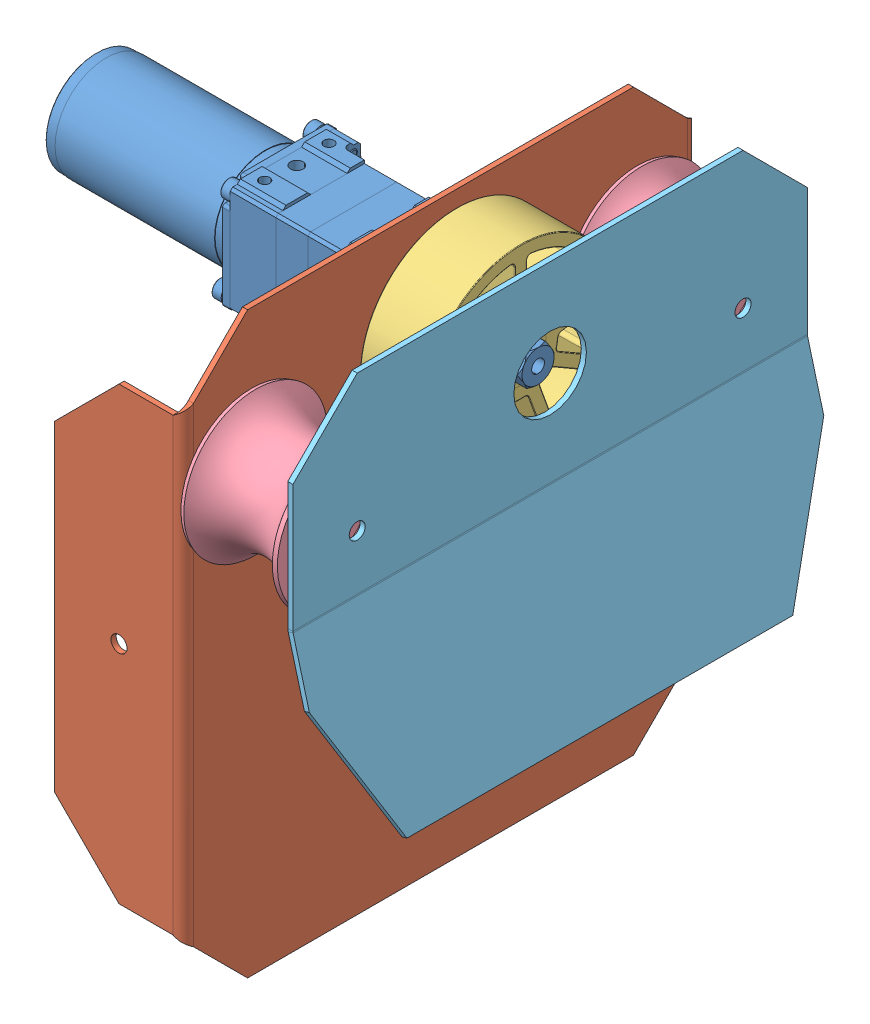
SolidWorks assembly ClimberCarriage, configuration Default. Lengths in mm.
Overall size (200.52 228.6 209.09).
7 component instances, 5 part files, 0 mates.
Components (placement in the parent):
- ClimberCarriage.stp-1: ClimberCarriage.stp [Default] at origin size (200.52 228.6 209.09)
  - VersaPlanetary_v2_Two_Stage_100_1_with_BAG.stp-1: VersaPlanetary_v2_Two_Stage_100_1_with_BAG.stp [Default] at (21.2553 -14.5157 8.7667) size (176.1 61.1 60.2)
  - Motor Side Plate 2.stp-1: Motor Side Plate 2.stp [Default] at (37.8803 29.9343 30.9917) x (0 1 0) z (1 0 0) size (228.6 203.3 50.85)
  - am-3945 3IN 500Hex Compliant Wheel VER 3.stp-1: am-3945 3IN 500Hex Compliant Wheel VER 3.stp [Default] at (87.5274 3.733 68.0189) x (0 0 1) z (-1 0 0) size (76.2 76.2 25.4)
  - Pulley2.stp-1: Pulley2.stp [Default] at (41.4998 -68.4907 8.7667) x (0 1 0) z (1 0 0) size (56.69 56.69 38.1)
  - Pulley2.stp-2: Pulley2.stp [Default] at (41.4998 -68.4907 -143.6333) x (0 1 0) z (1 0 0) size (56.69 56.69 38.1)
  - OutsidePlate2.stp-1: OutsidePlate2.stp [Default] at (81.1873 -68.4907 8.7667) x (0 1 0) z (1 0 0) size (149.8 203.2 21.68)
